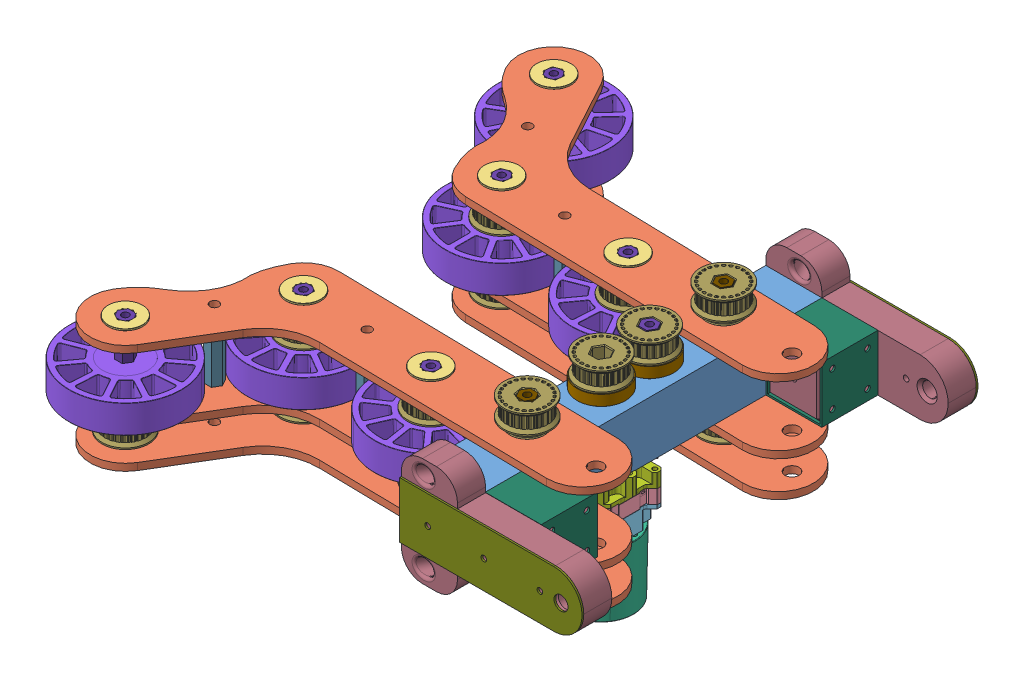
SolidWorks assembly Intake_Claw_1.0, configuration Default. Lengths in mm. (continued)
Mates (geometry in assembly coordinates): (continued)
- Coincident48: coincident anti-aligned: plane of 18_tooth_5mmHTD_timing_belt_pulley_9mm-1 through (25.4 82.7278 130.556) normal (0 1 0); plane of half_inch_hex_collar-2 through (25.4 82.7278 130.556) normal (0 -1 0)
- Concentric42: concentric aligned: circle of 18_tooth_5mmHTD_timing_belt_pulley_9mm-1; circle of half_inch_hex_collar-2
- Coincident50: coincident anti-aligned: plane of am-2986 FR8ZZ Hex Bearing.step-5 through (25.4 60.2513 225.7425) normal (0 1 0); plane of half_inch_hex_spacer_0.125inch-5 through (25.4 60.2513 241.3) normal (0 -1 0)
- Coincident51: coincident aligned: plane of Intake_Plate_Assembly_2-2/am-2986 FR8ZZ Hex Bearing.step-16 through (23.441 60.2513 78.9337) normal (0 1 0); circle of half_inch_hex_spacer_0.125inch-6
- Concentric43: concentric aligned: circle of Intake_Plate_Assembly_2-2/am-2986 FR8ZZ Hex Bearing.step-16; circle of half_inch_hex_spacer_0.125inch-6
- Concentric44: concentric aligned: circle of am-2986 FR8ZZ Hex Bearing.step-5; circle of half_inch_hex_spacer_0.125inch-5
- Coincident52: coincident anti-aligned: plane of am-2986 FR8ZZ Hex Bearing.step-5 through (25.4 60.2513 225.7425) normal (0 1 0); plane of half_inch_hex_spacer_0.1875inch-2 through (25.4 60.2513 241.3) normal (0 -1 0)
- Concentric45: concentric aligned: circle of am-2986 FR8ZZ Hex Bearing.step-5; circle of half_inch_hex_spacer_0.1875inch-2
- Coincident54: coincident anti-aligned: plane of Intake_Plate_Assembly_2-2/am-2986 FR8ZZ Hex Bearing.step-16 through (23.441 60.2513 78.9337) normal (0 1 0); plane of half_inch_hex_spacer_0.1875inch-1 through (25.4 60.2513 63.5) normal (0 -1 0)
- Concentric47: concentric aligned: circle of Intake_Plate_Assembly_2-2/am-2986 FR8ZZ Hex Bearing.step-16; circle of half_inch_hex_spacer_0.1875inch-1
- Concentric55: concentric aligned: circle of am-2986 FR8ZZ Hex Bearing.step-3; circle of 24_tooth_5mmHTD_timing_belt_pulley_9mm-2
- Concentric56: concentric aligned: cylinder of am-2986 FR8ZZ Hex Bearing.step-12 through (-180.9398 60.2513 237.4866) axis (0 -1 0) radius 15.5575; circle of 24_tooth_5mmHTD_timing_belt_pulley_9mm-3
- Concentric57: concentric aligned: circle of am-2986 FR8ZZ Hex Bearing.step-11; circle of 24_tooth_5mmHTD_timing_belt_pulley_9mm-4
- Concentric58: concentric aligned: circle of Intake_Plate_Assembly_2-2/am-2986 FR8ZZ Hex Bearing.step-18; circle of 24_tooth_5mmHTD_timing_belt_pulley_9mm-6
- Concentric59: concentric aligned: circle of Intake_Plate_Assembly_2-2/am-2986 FR8ZZ Hex Bearing.step-17; circle of 24_tooth_5mmHTD_timing_belt_pulley_9mm-5
- Concentric60: concentric anti-aligned: circle of Intake_Plate_Assembly_2-2/am-2986 FR8ZZ Hex Bearing.step-11; circle of 24_tooth_5mmHTD_timing_belt_pulley_9mm-1
- Coincident58: coincident anti-aligned: plane of half_inch_hex_spacer_0.1875inch-2 through (25.4 65.0138 241.3) normal (0 1 0); plane of 24_tooth_5mmHTD_timing_belt_pulley_9mm-7 through (25.4 65.0138 241.3) normal (0 -1 0)
- Concentric61: concentric anti-aligned: circle of half_inch_hex_spacer_0.1875inch-2; circle of 24_tooth_5mmHTD_timing_belt_pulley_9mm-7
- Coincident59: coincident anti-aligned: plane of Claw_Drive_Gear-2 through (25.4 64.9478 174.244) normal (0 1 0); plane of 24_tooth_5mmHTD_timing_belt_pulley_9mm-8 through (25.4 64.9478 174.244) normal (0 -1 0)
- Coincident60: coincident anti-aligned: plane of Claw_Drive_Gear-1 through (25.4 64.9478 130.556) normal (0 1 0); plane of 24_tooth_5mmHTD_timing_belt_pulley_9mm-9 through (25.4 64.9478 130.556) normal (0 -1 0)
- Concentric62: concentric anti-aligned: circle of Claw_Drive_Gear-1; circle of 24_tooth_5mmHTD_timing_belt_pulley_9mm-9
- Concentric63: concentric anti-aligned: circle of Claw_Drive_Gear-2; circle of 24_tooth_5mmHTD_timing_belt_pulley_9mm-8
- Coincident61: coincident anti-aligned: plane of half_inch_hex_spacer_0.1875inch-1 through (25.4 65.0138 63.5) normal (0 1 0); plane of 24_tooth_5mmHTD_timing_belt_pulley_9mm-10 through (25.4 65.0138 63.5) normal (0 -1 0)
- Concentric64: concentric anti-aligned: circle of half_inch_hex_spacer_0.1875inch-1; circle of 24_tooth_5mmHTD_timing_belt_pulley_9mm-10
- Coincident62: coincident aligned: circle of 24_tooth_5mmHTD_timing_belt_pulley_9mm-4; circle of 24_tooth_5mmHTD_timing_belt_pulley_9mm-11
- Concentric65: concentric anti-aligned: circle of Intake_Plate_Assembly_2-2/am-2986 FR8ZZ Hex Bearing.step-17; circle of 24_tooth_5mmHTD_timing_belt_pulley_9mm-5
- Concentric66: concentric anti-aligned: circle of Intake_Plate_Assembly_2-2/am-2986 FR8ZZ Hex Bearing.step-17; circle of 24_tooth_5mmHTD_timing_belt_pulley_9mm-13
- Concentric67: concentric anti-aligned: circle of am-2986 FR8ZZ Hex Bearing.step-12; circle of 24_tooth_5mmHTD_timing_belt_pulley_9mm-14
- Concentric68: concentric anti-aligned: circle of Intake_Plate_Assembly_2-2/am-2986 FR8ZZ Hex Bearing.step-11; circle of 24_tooth_5mmHTD_timing_belt_pulley_9mm-16
- Concentric69: concentric anti-aligned: circle of am-2986 FR8ZZ Hex Bearing.step-11; circle of 24_tooth_5mmHTD_timing_belt_pulley_9mm-15
- Coincident66: coincident anti-aligned: plane of am-3480 4IN 500Hex Bore Compliant Wheel REV2.STEP-4 through (-63.6188 27.051 63.7268) normal (0 1 0); plane of 24_tooth_5mmHTD_timing_belt_pulley_9mm-16 through (-63.47 27.051 61.1912) normal (0 -1 0)
- Coincident67: coincident anti-aligned: plane of am-3480 4IN 500Hex Bore Compliant Wheel REV2.STEP-3 through (-65.6418 27.051 238.316) normal (0 1 0); plane of 24_tooth_5mmHTD_timing_belt_pulley_9mm-15 through (-63.4848 27.051 239.6573) normal (0 -1 0)
- Coincident68: coincident anti-aligned: plane of am-3480 4IN 500Hex Bore Compliant Wheel REV2.STEP-5 through (-180.9054 27.051 60.6803) normal (0 1 0); plane of 24_tooth_5mmHTD_timing_belt_pulley_9mm-13 through (-180.9054 27.051 58.1403) normal (0 -1 0)
- Coincident69: coincident anti-aligned: plane of am-3480 4IN 500Hex Bore Compliant Wheel REV2.STEP-2 through (-178.7456 27.051 238.7661) normal (0 1 0); plane of 24_tooth_5mmHTD_timing_belt_pulley_9mm-3 through (-180.9398 27.051 237.4866) normal (0 -1 0)
- Coincident70: coincident anti-aligned: plane of am-3480 4IN 500Hex Bore Compliant Wheel REV2.STEP-4 through (-64.6717 1.651 81.6675) normal (0 -1 0); plane of half_inch_hex_spacer_0.125inch-13 through (-63.47 1.651 61.1912) normal (0 1 0)
- Coincident71: coincident anti-aligned: plane of Intake_Plate_Assembly-1/am-2986 FR8ZZ Hex Bearing.step-11 through (-63.47 -1.524 61.1912) normal (0 1 0); plane of half_inch_hex_spacer_0.125inch-13 through (-63.47 -1.524 61.1912) normal (0 -1 0)
- Concentric70: concentric aligned: cone of Intake_Plate_Assembly-1/am-2986 FR8ZZ Hex Bearing.step-11 through (-63.47 -7.9273 61.1912) axis (0 1 0); circle of half_inch_hex_spacer_0.125inch-13
- Coincident73: coincident anti-aligned: plane of am-3480 4IN 500Hex Bore Compliant Wheel REV2.STEP-5 through (-180.9054 1.651 78.6518) normal (0 -1 0); plane of half_inch_hex_spacer_0.125inch-14 through (-180.9054 1.651 58.1403) normal (0 1 0)
- Concentric71: concentric aligned: circle of am-3480 4IN 500Hex Bore Compliant Wheel REV2.STEP-5; circle of half_inch_hex_spacer_0.125inch-14
- Coincident74: coincident anti-aligned: plane of am-3480 4IN 500Hex Bore Compliant Wheel REV2.STEP-6 through (-217.1363 1.651 -50.2749) normal (0 -1 0); circle of half_inch_hex_spacer_0.125inch-15
- Concentric72: concentric aligned: circle of am-3480 4IN 500Hex Bore Compliant Wheel REV2.STEP-6; circle of half_inch_hex_spacer_0.125inch-15
- Coincident75: coincident anti-aligned: plane of am-3480 4IN 500Hex Bore Compliant Wheel REV2.STEP-3 through (-80.9029 1.651 228.8254) normal (0 -1 0); plane of half_inch_hex_spacer_0.125inch-16 through (-63.4848 1.651 239.6573) normal (0 1 0)
- Concentric73: concentric aligned: circle of am-3480 4IN 500Hex Bore Compliant Wheel REV2.STEP-3; circle of half_inch_hex_spacer_0.125inch-16
- Coincident76: coincident anti-aligned: plane of am-3480 4IN 500Hex Bore Compliant Wheel REV2.STEP-2 through (-163.2208 1.651 247.8191) normal (0 -1 0); plane of half_inch_hex_spacer_0.125inch-17 through (-180.9398 1.651 237.4866) normal (0 1 0)
- Concentric74: concentric aligned: circle of am-3480 4IN 500Hex Bore Compliant Wheel REV2.STEP-2; circle of half_inch_hex_spacer_0.125inch-17
- Coincident77: coincident anti-aligned: plane of am-3480 4IN 500Hex Bore Compliant Wheel REV2.STEP-1 through (-231.5582 1.651 356.0351) normal (0 -1 0); plane of half_inch_hex_spacer_0.125inch-18 through (-241.5471 1.651 338.1202) normal (0 1 0)
- Concentric75: concentric aligned: cylinder of am-3480 4IN 500Hex Bore Compliant Wheel REV2.STEP-1 through (-241.5471 -28.1452 338.1202) axis (0 1 0) radius 50.8; circle of half_inch_hex_spacer_0.125inch-18
- Coincident78: coincident anti-aligned: plane of am-2986 FR8ZZ Hex Bearing.step-3 through (-241.5471 60.2513 322.5627) normal (0 1 0); plane of half_inch_hex_spacer_0.125inch-9 through (-230.4157 60.2513 364.5609) normal (0 -1 0)
- Concentric76: concentric anti-aligned: circle of am-2986 FR8ZZ Hex Bearing.step-3; circle of half_inch_hex_spacer_0.125inch-9
- Coincident79: coincident aligned: plane of am-2986 FR8ZZ Hex Bearing.step-12 through (-180.9398 60.2513 221.9291) normal (0 1 0); circle of half_inch_hex_spacer_0.125inch-10
- Concentric77: concentric anti-aligned: circle of am-2986 FR8ZZ Hex Bearing.step-12; circle of half_inch_hex_spacer_0.125inch-10
- Coincident80: coincident anti-aligned: plane of am-2986 FR8ZZ Hex Bearing.step-11 through (-63.4848 60.2513 224.0998) normal (0 1 0); plane of half_inch_hex_spacer_0.125inch-12 through (-63.197 60.2513 248.6341) normal (0 -1 0)
- Concentric78: concentric anti-aligned: circle of am-2986 FR8ZZ Hex Bearing.step-11; circle of half_inch_hex_spacer_0.125inch-12
- Coincident81: coincident anti-aligned: plane of 24_tooth_5mmHTD_timing_belt_pulley_9mm-4 through (-63.197 63.4263 248.6341) normal (0 -1 0); circle of half_inch_hex_spacer_0.125inch-12
- Coincident83: coincident anti-aligned: plane of 24_tooth_5mmHTD_timing_belt_pulley_9mm-2 through (-230.4157 63.4263 364.5609) normal (0 -1 0); plane of half_inch_hex_spacer_0.125inch-9 through (-230.4157 63.4263 364.5609) normal (0 1 0)
- Coincident84: coincident anti-aligned: plane of 24_tooth_5mmHTD_timing_belt_pulley_9mm-14 through (-180.2715 63.4263 258.3256) normal (0 -1 0); plane of half_inch_hex_spacer_0.125inch-10 through (-180.2715 63.4263 258.3256) normal (0 1 0)
- Coincident85: coincident anti-aligned: plane of Intake_Plate_Assembly_2-2/am-2986 FR8ZZ Hex Bearing.step-11 through (-65.429 60.2513 76.6249) normal (0 1 0); plane of half_inch_hex_spacer_0.125inch-11 through (-63.3778 60.2513 58.8404) normal (0 -1 0)
- Concentric79: concentric anti-aligned: circle of Intake_Plate_Assembly_2-2/am-2986 FR8ZZ Hex Bearing.step-11; circle of half_inch_hex_spacer_0.125inch-11
- Coincident86: coincident anti-aligned: plane of 24_tooth_5mmHTD_timing_belt_pulley_9mm-12 through (-63.3778 63.4263 58.8404) normal (0 -1 0); plane of half_inch_hex_spacer_0.125inch-11 through (-63.3778 63.4263 58.8404) normal (0 1 0)
- Coincident87: coincident anti-aligned: plane of Intake_Plate_Assembly_2-2/am-2986 FR8ZZ Hex Bearing.step-18 through (-238.9399 60.2513 -29.6536) normal (0 1 0); plane of half_inch_hex_spacer_0.125inch-8 through (-234.0156 60.2513 -51.9922) normal (0 -1 0)
- Concentric80: concentric anti-aligned: circle of Intake_Plate_Assembly_2-2/am-2986 FR8ZZ Hex Bearing.step-18; circle of half_inch_hex_spacer_0.125inch-8
- Coincident88: coincident anti-aligned: plane of 24_tooth_5mmHTD_timing_belt_pulley_9mm-6 through (-234.0156 63.4263 -51.9922) normal (0 -1 0); plane of half_inch_hex_spacer_0.125inch-8 through (-234.0156 63.4263 -51.9922) normal (0 1 0)
- Coincident89: coincident anti-aligned: plane of Intake_Plate_Assembly_2-2/am-2986 FR8ZZ Hex Bearing.step-17 through (-182.8644 60.2513 73.5739) normal (0 1 0); plane of half_inch_hex_spacer_0.125inch-7 through (-180.6913 60.2513 52.683) normal (0 -1 0)
- Concentric81: concentric aligned: circle of Intake_Plate_Assembly_2-2/am-2986 FR8ZZ Hex Bearing.step-17; circle of half_inch_hex_spacer_0.125inch-7
- Coincident90: coincident anti-aligned: plane of 24_tooth_5mmHTD_timing_belt_pulley_9mm-5 through (-180.6913 63.4263 52.683) normal (0 -1 0); plane of half_inch_hex_spacer_0.125inch-7 through (-180.6913 63.4263 52.683) normal (0 1 0)
- Coincident95: coincident anti-aligned: plane of Claw_Crossbar-1 through (0 0 0) normal (0 0 -1); plane of Grabber_Spring_Mount-2 through (31.75 -4.7625 0) normal (0 0 1)
- Coincident97: coincident aligned: plane of Claw_Crossbar-1 through (50.8 0 304.8) normal (1 0 0); plane of Grabber_Spring_Mount-2 through (50.8 55.1815 -25.4) normal (1 0 0)
- Coincident101: coincident anti-aligned: plane of Intake_Plate_Assembly-1/am-2986 FR8ZZ Hex Bearing.step-5 through (23.441 -9.4513 78.9337) normal (0 -1 0); plane of half_inch_hex_spacer_0.125inch-19 through (25.4 -9.4513 63.5) normal (0 1 0)
- Concentric82: concentric anti-aligned: circle of Intake_Plate_Assembly-1/am-2986 FR8ZZ Hex Bearing.step-5; circle of half_inch_hex_spacer_0.125inch-19
- Coincident102: coincident anti-aligned: plane of 24_tooth_5mmHTD_timing_belt_pulley_9mm-18 through (25.4 -12.6263 63.5) normal (0 1 0); plane of half_inch_hex_spacer_0.125inch-19 through (25.4 -12.6263 63.5) normal (0 -1 0)
- Concentric83: concentric aligned: cylinder of 24_tooth_5mmHTD_timing_belt_pulley_9mm-18 through (25.4 -30.4063 63.5) axis (0 1 0) radius 21.082; circle of half_inch_hex_spacer_0.125inch-19
- Coincident103: coincident anti-aligned: plane of Intake_Plate_Assembly_2-1/am-2986 FR8ZZ Hex Bearing.step-16 through (24.1288 -9.4513 225.7945) normal (0 -1 0); plane of half_inch_hex_spacer_0.125inch-20 through (25.4 -9.4513 241.3) normal (0 1 0)
- Concentric84: concentric aligned: circle of Intake_Plate_Assembly_2-1/am-2986 FR8ZZ Hex Bearing.step-16; circle of half_inch_hex_spacer_0.125inch-20
- Coincident104: coincident anti-aligned: plane of 24_tooth_5mmHTD_timing_belt_pulley_9mm-17 through (25.4 -12.6263 241.3) normal (0 1 0); plane of half_inch_hex_spacer_0.125inch-20 through (25.4 -12.6263 241.3) normal (0 -1 0)
- Concentric85: concentric anti-aligned: circle of 24_tooth_5mmHTD_timing_belt_pulley_9mm-17; circle of half_inch_hex_spacer_0.125inch-20
- Coincident105: coincident anti-aligned: plane of Intake_Plate_Assembly-1/am-2986 FR8ZZ Hex Bearing.step-11 through (-65.429 -9.4513 76.6249) normal (0 -1 0); plane of half_inch_hex_spacer_0.125inch-21 through (-63.47 -9.4513 61.1912) normal (0 1 0)
- Concentric86: concentric anti-aligned: circle of Intake_Plate_Assembly-1/am-2986 FR8ZZ Hex Bearing.step-11; circle of half_inch_hex_spacer_0.125inch-21
- Coincident106: coincident anti-aligned: plane of half_inch_hex_spacer_0.125inch-21 through (-63.47 -12.6263 61.1912) normal (0 -1 0); plane of 24_tooth_5mmHTD_timing_belt_pulley_9mm-19 through (-63.47 -12.6263 61.1912) normal (0 1 0)
- Concentric87: concentric anti-aligned: circle of half_inch_hex_spacer_0.125inch-21; circle of 24_tooth_5mmHTD_timing_belt_pulley_9mm-19
- Coincident107: coincident anti-aligned: plane of half_inch_hex_spacer_0.125inch-30 through (-63.47 -30.4063 61.1912) normal (0 1 0); plane of 24_tooth_5mmHTD_timing_belt_pulley_9mm-19 through (-63.47 -30.4063 61.1912) normal (0 -1 0)
- Concentric88: concentric anti-aligned: circle of half_inch_hex_spacer_0.125inch-30; circle of 24_tooth_5mmHTD_timing_belt_pulley_9mm-19
- Coincident108: coincident anti-aligned: plane of Intake_Plate_Assembly-1/am-2986 FR8ZZ Hex Bearing.step-12 through (-182.8644 -9.4513 73.5739) normal (0 -1 0); plane of half_inch_hex_spacer_0.125inch-22 through (-180.9054 -9.4513 58.1403) normal (0 1 0)
- Concentric89: concentric anti-aligned: circle of Intake_Plate_Assembly-1/am-2986 FR8ZZ Hex Bearing.step-12; circle of half_inch_hex_spacer_0.125inch-22
- Coincident109: coincident anti-aligned: plane of half_inch_hex_spacer_0.125inch-22 through (-180.9054 -12.6263 58.1403) normal (0 -1 0); plane of 24_tooth_5mmHTD_timing_belt_pulley_9mm-20 through (-180.9054 -12.6263 58.1403) normal (0 1 0)
- Concentric90: concentric anti-aligned: circle of half_inch_hex_spacer_0.125inch-22; circle of 24_tooth_5mmHTD_timing_belt_pulley_9mm-20
- Coincident110: coincident anti-aligned: plane of half_inch_hex_spacer_0.125inch-31 through (-180.9054 -30.4063 58.1403) normal (0 1 0); plane of 24_tooth_5mmHTD_timing_belt_pulley_9mm-20 through (-180.9054 -30.4063 58.1403) normal (0 -1 0)
- Concentric91: concentric anti-aligned: circle of half_inch_hex_spacer_0.125inch-31; circle of 24_tooth_5mmHTD_timing_belt_pulley_9mm-20
- Coincident111: coincident anti-aligned: plane of Intake_Plate_Assembly-1/am-2986 FR8ZZ Hex Bearing.step-3 through (-238.9399 -9.4513 -29.6536) normal (0 -1 0); plane of half_inch_hex_spacer_0.125inch-23 through (-236.9809 -9.4513 -45.0872) normal (0 1 0)
- Concentric92: concentric anti-aligned: circle of Intake_Plate_Assembly-1/am-2986 FR8ZZ Hex Bearing.step-3; circle of half_inch_hex_spacer_0.125inch-23
- Coincident112: coincident anti-aligned: plane of half_inch_hex_spacer_0.125inch-23 through (-236.9809 -12.6263 -45.0872) normal (0 -1 0); plane of 24_tooth_5mmHTD_timing_belt_pulley_9mm-21 through (-236.9809 -12.6263 -45.0872) normal (0 1 0)
- Concentric93: concentric anti-aligned: circle of half_inch_hex_spacer_0.125inch-23; circle of 24_tooth_5mmHTD_timing_belt_pulley_9mm-21
- Coincident113: coincident anti-aligned: circle of half_inch_hex_spacer_0.125inch-32; plane of 24_tooth_5mmHTD_timing_belt_pulley_9mm-21 through (-236.9809 -30.4063 -45.0872) normal (0 -1 0)
- Concentric94: concentric anti-aligned: circle of half_inch_hex_spacer_0.125inch-32; circle of 24_tooth_5mmHTD_timing_belt_pulley_9mm-21
- Coincident114: coincident anti-aligned: plane of Intake_Plate_Assembly_2-1/am-2986 FR8ZZ Hex Bearing.step-18 through (-242.8184 -9.4513 322.6147) normal (0 -1 0); circle of half_inch_hex_spacer_0.125inch-24
- Concentric95: concentric anti-aligned: circle of Intake_Plate_Assembly_2-1/am-2986 FR8ZZ Hex Bearing.step-18; circle of half_inch_hex_spacer_0.125inch-24
- Coincident115: coincident anti-aligned: plane of half_inch_hex_spacer_0.125inch-24 through (-241.5471 -12.6263 338.1202) normal (0 -1 0); plane of 24_tooth_5mmHTD_timing_belt_pulley_9mm-22 through (-241.5471 -12.6263 338.1202) normal (0 1 0)
- Concentric96: concentric anti-aligned: circle of half_inch_hex_spacer_0.125inch-24; circle of 24_tooth_5mmHTD_timing_belt_pulley_9mm-22
- Coincident116: coincident anti-aligned: plane of half_inch_hex_spacer_0.125inch-29 through (-241.5471 -30.4063 338.1202) normal (0 1 0); plane of 24_tooth_5mmHTD_timing_belt_pulley_9mm-22 through (-241.5471 -30.4063 338.1202) normal (0 -1 0)
- Concentric97: concentric anti-aligned: circle of half_inch_hex_spacer_0.125inch-29; circle of 24_tooth_5mmHTD_timing_belt_pulley_9mm-22
- Coincident117: coincident anti-aligned: plane of Intake_Plate_Assembly_2-1/am-2986 FR8ZZ Hex Bearing.step-17 through (-182.211 -9.4513 221.9811) normal (0 -1 0); plane of half_inch_hex_spacer_0.125inch-25 through (-180.9398 -9.4513 237.4866) normal (0 1 0)
- Concentric98: concentric aligned: circle of Intake_Plate_Assembly_2-1/am-2986 FR8ZZ Hex Bearing.step-17; circle of half_inch_hex_spacer_0.125inch-25
- Coincident118: coincident anti-aligned: plane of half_inch_hex_spacer_0.125inch-25 through (-180.9398 -12.6263 237.4866) normal (0 -1 0); plane of 24_tooth_5mmHTD_timing_belt_pulley_9mm-23 through (-180.9398 -12.6263 237.4866) normal (0 1 0)
- Concentric99: concentric anti-aligned: circle of half_inch_hex_spacer_0.125inch-25; circle of 24_tooth_5mmHTD_timing_belt_pulley_9mm-23
- Coincident119: coincident anti-aligned: plane of half_inch_hex_spacer_0.125inch-28 through (-180.9398 -30.4063 237.4866) normal (0 1 0); plane of 24_tooth_5mmHTD_timing_belt_pulley_9mm-23 through (-180.9398 -30.4063 237.4866) normal (0 -1 0)
- Concentric100: concentric anti-aligned: circle of half_inch_hex_spacer_0.125inch-28; circle of 24_tooth_5mmHTD_timing_belt_pulley_9mm-23
- Coincident120: coincident anti-aligned: plane of Intake_Plate_Assembly_2-1/am-2986 FR8ZZ Hex Bearing.step-11 through (-64.7561 -9.4513 224.1518) normal (0 -1 0); plane of half_inch_hex_spacer_0.125inch-26 through (-63.4848 -9.4513 239.6573) normal (0 1 0)
- Concentric101: concentric anti-aligned: circle of Intake_Plate_Assembly_2-1/am-2986 FR8ZZ Hex Bearing.step-11; circle of half_inch_hex_spacer_0.125inch-26
- Coincident121: coincident anti-aligned: plane of half_inch_hex_spacer_0.125inch-26 through (-63.4848 -12.6263 239.6573) normal (0 -1 0); plane of 24_tooth_5mmHTD_timing_belt_pulley_9mm-24 through (-63.4848 -12.6263 239.6573) normal (0 1 0)
- Concentric102: concentric aligned: circle of Intake_Plate_Assembly_2-1/am-2986 FR8ZZ Hex Bearing.step-11; circle of 24_tooth_5mmHTD_timing_belt_pulley_9mm-24
- Coincident122: coincident anti-aligned: plane of half_inch_hex_spacer_0.125inch-27 through (-63.4848 -30.4063 239.6573) normal (0 1 0); plane of 24_tooth_5mmHTD_timing_belt_pulley_9mm-24 through (-63.4848 -30.4063 239.6573) normal (0 -1 0)
- Concentric103: concentric anti-aligned: circle of half_inch_hex_spacer_0.125inch-27; circle of 24_tooth_5mmHTD_timing_belt_pulley_9mm-24
- Coincident123: coincident anti-aligned: plane of 24_tooth_5mmHTD_timing_belt_pulley_9mm-18 through (25.4 -30.4063 63.5) normal (0 -1 0); plane of half_inch_hex_spacer_0.125inch-33 through (25.4 -30.4063 63.5) normal (0 1 0)
- Concentric104: concentric anti-aligned: circle of 24_tooth_5mmHTD_timing_belt_pulley_9mm-18; circle of half_inch_hex_spacer_0.125inch-33
- Coincident124: coincident anti-aligned: plane of 24_tooth_5mmHTD_timing_belt_pulley_9mm-17 through (25.4 -30.4063 241.3) normal (0 -1 0); plane of half_inch_hex_spacer_0.125inch-34 through (25.4 -30.4063 241.3) normal (0 1 0)
- Concentric105: concentric anti-aligned: circle of 24_tooth_5mmHTD_timing_belt_pulley_9mm-17; circle of half_inch_hex_spacer_0.125inch-34
- Coincident125: coincident anti-aligned: plane of half_inch_hex_spacer_0.125inch-27 through (-63.4848 -33.5813 239.6573) normal (0 -1 0); plane of Intake_Plate_Assembly_2-4/am-2986 FR8ZZ Hex Bearing.step-11 through (-63.4848 -33.5813 239.6573) normal (0 1 0)
- Concentric106: concentric aligned: circle of 24_tooth_5mmHTD_timing_belt_pulley_9mm-17; circle of Intake_Plate_Assembly_2-4/am-2986 FR8ZZ Hex Bearing.step-16
- Coincident126: coincident aligned: plane of Intake_Plate_Assembly_2-1/Claw_Intake_Plates-3 through (75.6047 -1.5773 273.9833) normal (-0.018478 0 0.999829); plane of Intake_Plate_Assembly_2-4/Claw_Intake_Plates-3 through (75.6047 -33.6347 273.9833) normal (-0.018478 0 0.999829)
- Coincident127: coincident anti-aligned: plane of half_inch_hex_spacer_0.125inch-33 through (25.4 -33.5813 63.5) normal (0 -1 0); plane of Intake_Plate_Assembly-3/am-2986 FR8ZZ Hex Bearing.step-5 through (25.4 -33.5813 63.5) normal (0 1 0)
- Concentric107: concentric anti-aligned: circle of half_inch_hex_spacer_0.125inch-33; circle of Intake_Plate_Assembly-3/am-2986 FR8ZZ Hex Bearing.step-5
- Coincident128: coincident aligned: plane of Intake_Plate_Assembly-1/Claw_Intake_Plates-3 through (77.0074 -7.9273 33.08) normal (0.025971 0 -0.999663); plane of Intake_Plate_Assembly-3/Claw_Intake_Plates-3 through (77.0074 -39.9847 33.08) normal (0.025971 0 -0.999663)
- Coincident130: coincident anti-aligned: plane of Intake_Plate_Assembly_2-1/Claw_Intake_Plates-3 through (-241.5471 -1.5773 338.1202) normal (0 1 0); plane of grabber_stand_off-1 through (-122.2123 -1.5773 238.572) normal (0 -1 0)
- Concentric109: concentric anti-aligned: circle of Claw_Intake_Plates-3; circle of grabber_stand_off-1
- Coincident132: coincident anti-aligned: plane of Claw_Intake_Plates-3 through (-241.5471 52.3773 338.1202) normal (0 -1 0); plane of grabber_stand_off-3 through (-211.2434 52.3773 287.8034) normal (0 1 0)
- Concentric110: concentric anti-aligned: circle of Claw_Intake_Plates-3; circle of grabber_stand_off-3
- Coincident133: coincident anti-aligned: plane of Intake_Plate_Assembly_2-2/Claw_Intake_Plates-3 through (-236.9809 52.3773 -45.0872) normal (0 -1 0); plane of grabber_stand_off-5 through (-122.1877 52.3773 59.6657) normal (0 1 0)
- Concentric111: concentric aligned: circle of Intake_Plate_Assembly_2-2/Claw_Intake_Plates-3; circle of grabber_stand_off-5
- Coincident134: coincident anti-aligned: plane of Intake_Plate_Assembly_2-2/Claw_Intake_Plates-3 through (-236.9809 52.3773 -45.0872) normal (0 -1 0); plane of grabber_stand_off-4 through (-208.9431 52.3773 6.5265) normal (0 1 0)
- Concentric112: concentric aligned: circle of Intake_Plate_Assembly_2-2/Claw_Intake_Plates-3; circle of grabber_stand_off-4
- Coincident136: coincident anti-aligned: plane of Claw_Crossbar-1 through (1.5875 1.5875 304.8) normal (0 1 0); plane of Grabber_Spring_Mount-2 through (48.8315 1.5875 0) normal (0 -1 0)
- Coincident137: coincident anti-aligned: plane of Claw_Crossbar-1 through (1.5875 1.5875 304.8) normal (0 1 0); plane of Grabber_Spring_Mount-1 through (49.2125 1.5875 304.8) normal (0 -1 0)
- Coincident138: coincident anti-aligned: plane of Claw_Crossbar-1 through (49.2125 1.5875 304.8) normal (-1 0 0); plane of Grabber_Spring_Mount-1 through (49.2125 48.8315 304.8) normal (1 0 0)
- Coincident139: coincident anti-aligned: plane of Claw_Crossbar-1 through (0 0 304.8) normal (0 0 1); plane of Grabber_Spring_Mount-1 through (32.131 55.1815 304.8) normal (0 0 -1)
- Coincident140: coincident aligned: plane of Claw_Crossbar-1 through (0 0 304.8) normal (0 -1 0); plane of Crossbar_Bracket-1 through (101.6 0 50.8) normal (0 -1 0)
- Coincident141: coincident anti-aligned: plane of Claw_Crossbar-1 through (50.8 0 304.8) normal (1 0 0); plane of Crossbar_Bracket-1 through (50.8 0 50.8) normal (-1 0 0)
- Coincident142: coincident: line of Claw_Crossbar-1 through (0 50.8 0) axis (0 0 1); plane of Crossbar_Bracket-1 through (101.6 0 0) normal (0 0 -1)
- Coincident143: coincident anti-aligned: plane of Claw_Crossbar-1 through (50.8 0 304.8) normal (1 0 0); plane of Crossbar_Bracket-2 through (50.8 0 304.8) normal (-1 0 0)
- Coincident144: coincident aligned: plane of Claw_Crossbar-1 through (0 0 304.8) normal (0 -1 0); plane of Crossbar_Bracket-2 through (101.6 0 304.8) normal (0 -1 0)
- Coincident145: coincident: plane of Claw_Crossbar-1; plane of Crossbar_Bracket-2 through (101.6 0 304.8) normal (0 0 1)
- Coincident146: coincident anti-aligned: plane of Grabber_Spring_Mount-1 through (32.131 55.1815 330.2) normal (0 0 1); plane of Claw_Pivot_Plate-1 through (140.081 25.2095 330.2) normal (0 0 -1)
- Concentric114: concentric anti-aligned: circle of Grabber_Spring_Mount-1; circle of Claw_Pivot_Plate-1
- Coincident147: coincident anti-aligned: plane of Grabber_Spring_Mount-2 through (31.75 -4.7625 -25.4) normal (0 0 -1); plane of Claw_Pivot_Plate-2 through (139.7 25.2095 -25.4) normal (0 0 1)
- Concentric115: concentric aligned: circle of Grabber_Spring_Mount-2; circle of Claw_Pivot_Plate-2
- Coincident148: coincident aligned: plane of Grabber_Spring_Mount-2 through (165.1 -0.1905 0) normal (0 -1 0); plane of Claw_Pivot_Plate-2 through (0 -0.1905 -25.4) normal (0 -1 0)
- Coincident149: coincident aligned: plane of Grabber_Spring_Mount-1 through (165.481 -0.1905 304.8) normal (0 -1 0); plane of Claw_Pivot_Plate-1 through (0.381 -0.1905 331.7875) normal (0 -1 0)
- Concentric116: concentric aligned: circle of Intake_Plate_Assembly-3/am-2986 FR8ZZ Hex Bearing.step-3; circle of grabber_wheel_axle-1
- Coincident151: coincident aligned: plane of Intake_Plate_Assembly_2-2/am-2986 FR8ZZ Hex Bearing.step-18 through (-238.9399 60.2513 -29.6536) normal (0 1 0); plane of grabber_wheel_axle-1 through (-236.9809 60.2513 -45.0872) normal (0 1 0)
- Concentric117: concentric aligned: circle of Intake_Plate_Assembly_2-2/am-2986 FR8ZZ Hex Bearing.step-17; circle of grabber_wheel_axle-2
- Coincident152: coincident aligned: plane of Intake_Plate_Assembly_2-2/am-2986 FR8ZZ Hex Bearing.step-17 through (-182.8644 60.2513 73.5739) normal (0 1 0); plane of grabber_wheel_axle-2 through (-180.9054 60.2513 58.1403) normal (0 1 0)
- Concentric118: concentric aligned: circle of Intake_Plate_Assembly_2-2/am-2986 FR8ZZ Hex Bearing.step-11; circle of grabber_wheel_axle-3
- Coincident153: coincident aligned: plane of Intake_Plate_Assembly_2-2/am-2986 FR8ZZ Hex Bearing.step-11 through (-65.429 60.2513 76.6249) normal (0 1 0); plane of grabber_wheel_axle-3 through (-63.47 60.2513 61.1912) normal (0 1 0)
- Coincident154: coincident aligned: plane of am-2986 FR8ZZ Hex Bearing.step-3 through (-241.5471 60.2513 322.5627) normal (0 1 0); plane of grabber_wheel_axle-5 through (-241.5471 60.2513 338.1202) normal (0 1 0)
- Concentric120: concentric anti-aligned: circle of am-2986 FR8ZZ Hex Bearing.step-3; circle of grabber_wheel_axle-5
- Coincident155: coincident aligned: plane of am-2986 FR8ZZ Hex Bearing.step-12 through (-180.9398 60.2513 221.9291) normal (0 1 0); plane of grabber_wheel_axle-6 through (-180.9398 60.2513 237.4866) normal (0 1 0)
- Concentric121: concentric anti-aligned: circle of am-2986 FR8ZZ Hex Bearing.step-12; circle of grabber_wheel_axle-6
- Concentric122: concentric anti-aligned: circle of am-2986 FR8ZZ Hex Bearing.step-11; circle of grabber_wheel_axle-7
- Coincident156: coincident aligned: plane of am-2986 FR8ZZ Hex Bearing.step-11 through (-63.4848 60.2513 224.0998) normal (0 1 0); plane of grabber_wheel_axle-7 through (-63.4848 60.2513 239.6573) normal (0 1 0)
- Coincident157: coincident aligned: plane of 24_tooth_5mmHTD_timing_belt_pulley_9mm-9 through (25.4 82.7278 130.556) normal (0 1 0); plane of grabber_wheel_axle-4 through (25.4 82.7278 130.556) normal (0 1 0)
- Concentric123: concentric aligned: circle of 24_tooth_5mmHTD_timing_belt_pulley_9mm-9; circle of grabber_wheel_axle-4
- Coincident158: coincident aligned: plane of 24_tooth_5mmHTD_timing_belt_pulley_9mm-10 through (25.4 82.7938 63.5) normal (0 1 0); plane of grabber_pivot_axle-1 through (25.4 82.7938 63.5) normal (0 1 0)
- Concentric124: concentric aligned: circle of 24_tooth_5mmHTD_timing_belt_pulley_9mm-10; circle of grabber_pivot_axle-1
- Coincident159: coincident anti-aligned: circle of 24_tooth_5mmHTD_timing_belt_pulley_9mm-7; plane of grabber_pivot_axle-2 through (25.4 82.7938 241.3) normal (0 1 0)
- Concentric125: concentric aligned: circle of 24_tooth_5mmHTD_timing_belt_pulley_9mm-7; circle of grabber_pivot_axle-2
